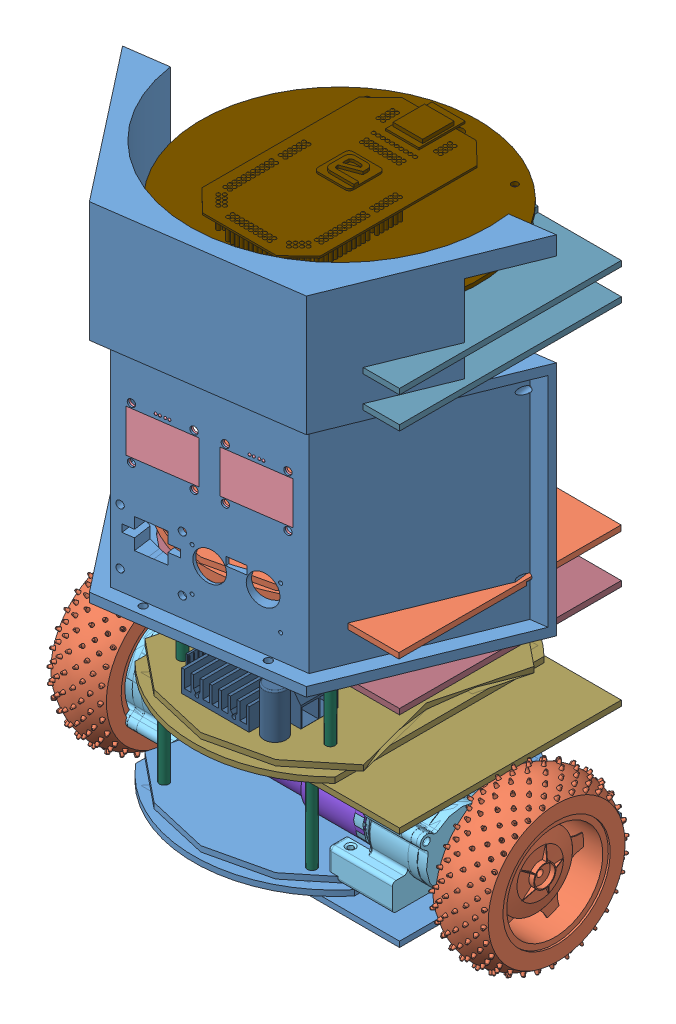
SolidWorks assembly Assembly_Final, configuration Default. Lengths in mm.
Overall size (236.68 351.62 182.38).
53 component instances, 26 part files, 124 mates.
Components (placement in the parent):
- BASE PLATE COMPACT-1: BASE PLATE COMPACT [Default] at (49.4415 46.8025 149.989) size (151.66 9 157.59)
- 85mm_Wheel-1: 85mm_Wheel [Default] at (-6.3675 60.3759 90.7884) x (0 -0.941771 -0.336255) z (0 0.336255 -0.941771) size (89.76 30.03 89.76)
- Bearing_large-1: Bearing_large [Default] at (14.6025 60.3759 90.7884) x (0 0 1) z (-1 0 0) size (34 34 10)
- Bearing_Modifiable-1: Bearing_Modifiable [Default] at (157.8505 60.3759 90.7897) x (0 0.995431 -0.095482) z (1 0 0) size (16 16 5)
- Gear Box Covering - Modifiable-1: Gear Box Covering - Modifiable [Default] at (31.0325 60.3759 90.7884) x (0 -0.541121 0.840945) z (-1 0 0) size (87.3 57.46 46.55)
- Gear_Driven - LARGE-1: Gear_Driven - LARGE [Default] at (169.8505 60.3759 90.7897) x (0 0.167526 -0.985868) z (1 0 0) size (41.92 41.92 47.93)
- Gear_Driver-1: Gear_Driver [Default] at (24.0325 76.7719 65.3077) x (0 0 1) z (-1 0 0) size (21.81 21.81 25.3)
- IG32 MOTORS-1: IG32 MOTORS [Default] at (41.0325 76.7719 65.3077) x (1 0 0) z (0 -1 0) size (92 51.5 40)
- LINE SENSOR-1: LINE SENSOR [Default] at (146.9415 49.8025 103.989) x (-1 0 0) z (0 0 1) size (100 13.5 28)
- Motor Driver-1: Motor Driver [Default] at (96.9415 105.8025 134.589) size (71 27 36.5)
- Motor_Main_Shaft-1: Motor_Main_Shaft [Default] at (41.0325 76.7719 65.3077) x (0 0 1) z (-1 0 0) size (6 6 15)
- Gear Box Covering - Modifiable-2: Gear Box Covering - Modifiable [Default] at (162.8505 60.3759 90.7897) x (0 -0.541121 -0.840945) z (1 0 0) size (87.3 57.46 46.55)
- Gear_Driver-2: Gear_Driver [Default] at (169.8505 76.7719 116.2703) x (0 -0.01238 -0.999923) z (1 0 0) size (21.81 21.81 25.3)
- Gear_Driven - LARGE-2: Gear_Driven - LARGE [Default] at (24.0325 60.3759 90.7884) x (0 0.762091 -0.64747) z (-1 0 0) size (41.92 41.92 47.93)
- IG32 MOTORS-2: IG32 MOTORS [Default] at (152.8505 76.7719 116.2703) x (-1 0 0) z (0 -1 0) size (92 51.5 40)
- Motor_Main_Shaft-2: Motor_Main_Shaft [Default] at (152.8505 76.7719 116.2703) x (0 -0.01238 -0.999923) z (1 0 0) size (6 6 15)
- Bearing_Modifiable-2: Bearing_Modifiable [Default] at (31.0325 60.3759 90.7884) x (0 0 -1) z (1 0 0) size (16 16 5)
- Bearing_Modifiable-3: Bearing_Modifiable [Default] at (14.6025 76.7719 65.3077) x (0 0 1) z (-1 0 0) size (16 16 5)
- Bearing_Modifiable-4: Bearing_Modifiable [Default] at (179.2805 76.7719 116.2703) x (0 0 -1) z (1 0 0) size (16 16 5)
- Bearing_large-2: Bearing_large [Default] at (179.2805 60.3759 90.7897) x (0 0 -1) z (1 0 0) size (34 34 10)
- 85mm_Wheel-2: 85mm_Wheel [Default] at (200.2505 60.3759 90.7897) x (0 0.770023 0.638016) z (0 0.638016 -0.770023) size (89.76 30.03 89.76)
- Floor_Plates1-1: Floor_Plates1 [Default] at (49.4415 99.8025 149.989) size (151.66 9 157.59)
- Floor_Plates2-1: Floor_Plates2 [Default] at (49.4415 155.8025 149.989) size (151.66 9 150)
- Floor_Plates4_2-1: Floor_Plates4_2 [Default] at (49.4415 288.8025 149.989) size (151.66 11 150)
- 3cm_spacers-1: 3cm_spacers [Default] at (56.9415 112.8025 144.839) x (0.995934 0 0.090084) z (0 -1 0) size (5 5 55)
- 3cm_spacers-2: 3cm_spacers [Default] at (56.9415 112.8025 35.139) x (0.477251 0 0.878767) z (0 -1 0) size (5 5 55)
- 3cm_spacers-3: 3cm_spacers [Default] at (136.9415 112.8025 144.839) x (0.906468 0 -0.422275) z (0 -1 0) size (5 5 55)
- 3cm_spacers-4: 3cm_spacers [Default] at (136.9415 112.8025 35.139) x (-0.928661 0 -0.370929) z (0 -1 0) size (5 5 55)
- 3cm_spacers-5: 3cm_spacers [Default] at (56.9415 165.8025 134.839) x (-0.9484 0 0.317076) z (0 -1 0) size (5 5 55)
- 3cm_spacers-6: 3cm_spacers [Default] at (136.9415 165.8025 45.139) x (0.243331 0 0.969943) z (0 -1 0) size (5 5 55)
- 3cm_spacers-7: 3cm_spacers [Default] at (56.9415 165.8025 45.139) x (0.021183 0 -0.999776) z (0 -1 0) size (5 5 55)
- 3cm_spacers-8: 3cm_spacers [Default] at (136.9007 165.8025 134.839) x (0.022963 0 -0.999736) z (0 -1 0) size (5 5 55)
- Motor Driver-2: Motor Driver [Default] at (96.9415 105.8025 45.389) size (71 27 36.5)
- 6cm_spacers-1: 6cm_spacers [Default] at (67.4804 303.8025 130.3876) x (-0.877081 0 0.480343) z (0 -1 0) size (5 5 150)
- 6cm_spacers-2: 6cm_spacers [Default] at (126.4026 303.8025 130.3876) x (-0.604095 0 0.796913) z (0 -1 0) size (5 5 150)
- 6cm_spacers-3: 6cm_spacers [Default] at (126.4026 303.8025 49.5905) x (0.449735 0 -0.893162) z (0 -1 0) size (5 5 150)
- 6cm_spacers-4: 6cm_spacers [Default] at (67.4804 303.8025 49.5905) x (-0.570107 0 0.82157) z (0 -1 0) size (5 5 150)
- Floor_Plates4_2-2: Floor_Plates4_2 [Default] at (49.4415 305.8025 149.989) size (151.66 11 150)
- spacer 2cm-2: spacer 2cm [Default] at (56.9415 318.8025 35.139) x (1 0 0) z (0 -1 0) size (5 5 15)
- spacer 2cm-3: spacer 2cm [Default] at (56.9415 318.8025 144.839) x (1 0 0) z (0 -1 0) size (5 5 15)
- spacer 2cm-4: spacer 2cm [Default] at (136.9415 318.8025 144.839) x (1 0 0) z (0 -1 0) size (5 5 15)
- spacer 2cm-5: spacer 2cm [Default] at (136.9415 318.8025 35.139) x (-0.160784 0 0.98699) z (0 -1 0) size (5 5 15)
- eYFi_Mega-2: eYFi_Mega [Default] at (76.9415 330.8025 143.989) size (150 18 150)
- Cover_mid-1: Cover_mid [Default] at (96.9415 158.8025 89.989) size (207.85 128 180) (hidden)
- Cover_Top-1: Cover_Top [Default] at (96.9415 336.8025 89.989) x (1 0 0) z (0 -1 0) size (207.85 180 50) (hidden)
- Cover_Bottom-1: Cover_Bottom [Default] at (96.9415 153.8025 89.989) size (205.85 109.54 180) (hidden)
- Cover_Bottom-2: Cover_Bottom [Default] at (96.9415 155.8025 89.989) x (0.990267 0 -0.139181) z (0.139181 0 0.990267) size (205.85 109.54 180) (hidden)
- Cover_Front-1: Cover_Front [Default] at (96.9415 160.8025 89.989) x (0.990267 0 -0.139181) z (0.139181 0 0.990267) size (207.85 188 90)
- Cover_Back-1: Cover_Back [Default] at (96.9415 160.8025 89.989) x (0.990267 0 -0.139181) z (0.139181 0 0.990267) size (207.85 188 90) (hidden)
- Dead_weight-1: Dead_weight [Default] at (49.303 182.022 149.8791) x (0.999997 0 0.002311) z (-0.002311 0 0.999997) size (151.66 12 150)
- Lead_Screw-1: Lead_Screw [Default] at (96.9415 158.8025 89.989) x (-0.659999 0 -0.751266) z (0.751266 0 -0.659999) size (7.8 150 7.8)
- OLED-2: OLED [Default] at (130.4266 242.3025 166.5739) x (0.990267 0 -0.139181) z (0.139181 0 0.990267) size (35 33 8.5)
- OLED-3: OLED [Default] at (85.8646 242.3025 172.8371) x (0.990267 0 -0.139181) z (0.139181 0 0.990267) size (35 33 8.5)
Mates (geometry in assembly coordinates):
- Coincident4: coincident anti-aligned: plane of BASE PLATE COMPACT-1 through (167.7549 49.8025 89.989) normal (0 -1 0); plane of LINE SENSOR-1 through (146.9415 49.8025 103.989) normal (0 1 0)
- Concentric1: concentric anti-aligned: cylinder of BASE PLATE COMPACT-1 through (49.4415 57.8025 101.489) axis (0 -1 0) radius 1.711; cylinder of LINE SENSOR-1 through (49.4415 47.8025 101.489) axis (0 1 0) radius 1.5
- Concentric2: concentric anti-aligned: cylinder of BASE PLATE COMPACT-1 through (144.4415 57.8025 101.489) axis (0 -1 0) radius 1.711; cylinder of LINE SENSOR-1 through (144.4415 47.8025 101.489) axis (0 1 0) radius 1.5
- Coincident9: coincident anti-aligned: plane of IG32 MOTORS-1 through (41.0325 76.7719 65.3077) normal (-1 0 0); plane of Motor_Main_Shaft-1 through (41.0325 76.7719 65.3077) normal (1 0 0)
- Concentric6: concentric aligned: cylinder of IG32 MOTORS-1 through (38.0325 76.7719 65.3077) axis (1 0 0) radius 10.5; cylinder of Motor_Main_Shaft-1 through (26.0325 76.7719 65.3077) axis (1 0 0) radius 3
- Coincident10: coincident anti-aligned: plane of IG32 MOTORS-2 through (152.8505 76.7719 116.2703) normal (1 0 0); plane of Motor_Main_Shaft-2 through (152.8505 76.7719 116.2703) normal (-1 0 0)
- Concentric7: concentric aligned: cylinder of IG32 MOTORS-2 through (155.8505 76.7719 116.2703) axis (-1 0 0) radius 10.5; cylinder of Motor_Main_Shaft-2 through (167.8505 76.7719 116.2703) axis (-1 0 0) radius 3
- Coincident11: coincident anti-aligned: plane of BASE PLATE COMPACT-1 through (167.7549 52.8025 89.989) normal (0 1 0); plane of Gear Box Covering - Modifiable-2 through (177.8505 52.8025 90.7897) normal (0 -1 0)
- Concentric8: concentric aligned: cylinder of BASE PLATE COMPACT-1 through (149.6005 41.8025 136.5916) axis (0 1 0) radius 1.75; cylinder of Gear Box Covering - Modifiable-2 through (149.6005 42.6025 136.5916) axis (0 1 0) radius 1.5
- Parallel5: parallel aligned: plane of BASE PLATE COMPACT-1 through (156.1015 49.8025 43.8903) normal (1 0 0); plane of Gear Box Covering - Modifiable-2 through (162.8505 76.7719 116.2703) normal (1 0 0)
- Coincident13: coincident anti-aligned: plane of BASE PLATE COMPACT-1 through (167.7549 52.8025 89.989) normal (0 1 0); plane of Gear Box Covering - Modifiable-1 through (16.0325 52.8025 90.7884) normal (0 -1 0)
- Concentric12: concentric aligned: cylinder of BASE PLATE COMPACT-1 through (44.2825 41.8025 44.9864) axis (0 1 0) radius 1.75; cylinder of Gear Box Covering - Modifiable-1 through (44.2825 42.6025 44.9864) axis (0 1 0) radius 1.5
- Parallel6: parallel aligned: plane of BASE PLATE COMPACT-1 through (37.7815 49.8025 43.8903) normal (-1 0 0); plane of Gear Box Covering - Modifiable-1 through (31.0325 76.7719 65.3077) normal (-1 0 0)
- Concentric13: concentric anti-aligned: cylinder of Gear Box Covering - Modifiable-2 through (167.8505 76.7719 116.2703) axis (-1 0 0) radius 10.75; cylinder of IG32 MOTORS-2 through (147.8505 76.7719 116.2703) axis (1 0 0) radius 16.5
- Concentric14: concentric aligned: cylinder of Gear Box Covering - Modifiable-2 through (157.8505 90.2719 116.2703) axis (1 0 0) radius 1.75; cylinder of IG32 MOTORS-2 through (149.8505 90.2719 116.2703) axis (1 0 0) radius 1.5
- Coincident16: coincident anti-aligned: plane of Gear Box Covering - Modifiable-2 through (152.8505 76.7719 116.2703) normal (-1 0 0); plane of IG32 MOTORS-2 through (152.8505 76.7719 116.2703) normal (1 0 0)
- Concentric15: concentric anti-aligned: cylinder of Gear Box Covering - Modifiable-1 through (26.0325 76.7719 65.3077) axis (1 0 0) radius 10.75; cylinder of IG32 MOTORS-1 through (46.0325 76.7719 65.3077) axis (-1 0 0) radius 16.5
- Concentric16: concentric aligned: cylinder of Gear Box Covering - Modifiable-1 through (36.0325 90.2719 65.3077) axis (-1 0 0) radius 1.75; cylinder of IG32 MOTORS-1 through (44.0325 90.2719 65.3077) axis (-1 0 0) radius 1.5
- Coincident17: coincident anti-aligned: plane of Gear Box Covering - Modifiable-1 through (41.0325 76.7719 65.3077) normal (1 0 0); plane of IG32 MOTORS-1 through (41.0325 76.7719 65.3077) normal (-1 0 0)
- Concentric17: concentric anti-aligned: cone of Gear_Driver-2 through (158.0485 76.7719 116.2703) axis (1 0 0); cylinder of Motor_Main_Shaft-2 through (167.8505 76.7719 116.2703) axis (-1 0 0) radius 3
- Concentric18: concentric anti-aligned: cylinder of Gear_Driver-2 through (161.8505 89.7709 116.1094) axis (0 -0.999923 0.01238) radius 2; cylinder of Motor_Main_Shaft-2 through (161.8505 73.2721 116.3136) axis (0 0.999923 -0.01238) radius 1.5
- Concentric19: concentric anti-aligned: cylinder of Gear_Driven - LARGE-1 through (154.9205 60.3759 90.7897) axis (1 0 0) radius 2.8; cylinder of Gear Box Covering - Modifiable-2 through (189.2805 60.3759 90.7897) axis (-1 0 0) radius 17.25
- Coincident18: coincident aligned: plane of Gear_Driven - LARGE-1 through (172.3505 60.3759 90.7897) normal (1 0 0); plane of Gear_Driver-2 through (172.3505 76.7719 116.2703) normal (1 0 0)
- Concentric20: concentric anti-aligned: cylinder of Gear_Driver-1 through (38.0325 76.7719 65.3077) axis (-1 0 0) radius 5.75; cylinder of Motor_Main_Shaft-1 through (26.0325 76.7719 65.3077) axis (1 0 0) radius 3
- Concentric21: concentric anti-aligned: cylinder of Gear_Driver-1 through (32.0325 89.7719 65.3077) axis (0 -1 0) radius 2; cylinder of Motor_Main_Shaft-1 through (32.0325 73.2719 65.3077) axis (0 1 0) radius 1.5
- Concentric24: concentric aligned: cylinder of Gear Box Covering - Modifiable-1 through (14.6025 60.3759 90.7884) axis (1 0 0) radius 22; cylinder of Gear_Driven - LARGE-2 through (-4.7675 60.3759 90.7884) axis (1 0 0) radius 7.5
- Coincident20: coincident aligned: plane of Gear_Driver-1 through (21.5325 76.7719 65.3077) normal (-1 0 0); plane of Gear_Driven - LARGE-2 through (21.5325 60.3759 90.7884) normal (-1 0 0)
- Concentric25: concentric anti-aligned: cylinder of Gear Box Covering - Modifiable-1 through (36.0325 60.3759 90.7884) axis (-1 0 0) radius 8.75; cylinder of Bearing_Modifiable-2 through (31.0325 60.3759 90.7884) axis (1 0 0) radius 8
- Coincident21: coincident aligned: plane of Gear Box Covering - Modifiable-1 through (31.0325 76.7719 65.3077) normal (-1 0 0); circle of Bearing_Modifiable-2
- Concentric27: concentric anti-aligned: cylinder of Gear Box Covering - Modifiable-1 through (9.6025 76.7719 65.3077) axis (1 0 0) radius 8.25; cylinder of Bearing_Modifiable-3 through (14.6025 76.7719 65.3077) axis (-1 0 0) radius 8
- Coincident22: coincident: line of Gear Box Covering - Modifiable-1 through (9.6025 62.7096 52.5308) axis (0 -0.672473 0.740122); plane of Bearing_Modifiable-3 through (9.6025 76.7719 65.3077) normal (-1 0 0)
- Concentric28: concentric anti-aligned: cylinder of Bearing_Modifiable-1 through (157.8505 60.3759 90.7897) axis (1 0 0) radius 8; cylinder of Gear Box Covering - Modifiable-2 through (189.2805 60.3759 90.7897) axis (-1 0 0) radius 17.25
- Coincident23: coincident aligned: plane of Bearing_Modifiable-1 through (162.8505 60.3759 90.7897) normal (1 0 0); plane of Gear Box Covering - Modifiable-2 through (162.8505 76.7719 116.2703) normal (1 0 0)
- Concentric30: concentric anti-aligned: cylinder of Gear Box Covering - Modifiable-2 through (184.2805 76.7719 116.2703) axis (-1 0 0) radius 8.25; cylinder of Bearing_Modifiable-4 through (179.2805 76.7719 116.2703) axis (1 0 0) radius 8
- Coincident25: coincident aligned: plane of Gear Box Covering - Modifiable-2 through (184.2805 83.1136 136.2899) normal (1 0 0); plane of Bearing_Modifiable-4 through (184.2805 76.7719 116.2703) normal (1 0 0)
- Concentric31: concentric anti-aligned: cylinder of Gear_Driven - LARGE-1 through (198.6505 60.3759 90.7897) axis (-1 0 0) radius 7.5; cylinder of Bearing_large-2 through (179.2805 60.3759 90.7897) axis (1 0 0) radius 17
- Coincident26: coincident aligned: plane of Gear Box Covering - Modifiable-2 through (189.2805 60.3759 90.7897) normal (1 0 0); plane of Bearing_large-2 through (189.2805 60.3759 90.7897) normal (1 0 0)
- Concentric32: concentric anti-aligned: cylinder of Bearing_large-1 through (14.6025 60.3759 90.7884) axis (-1 0 0) radius 17; cylinder of Gear_Driven - LARGE-2 through (-4.7675 60.3759 90.7884) axis (1 0 0) radius 7.5
- Coincident27: coincident aligned: plane of Bearing_large-1 through (4.6025 60.3759 90.7884) normal (-1 0 0); plane of Gear Box Covering - Modifiable-1 through (4.6025 60.3759 90.7884) normal (-1 0 0)
- Concentric33: concentric aligned: cylinder of Gear_Driven - LARGE-1 through (198.6505 60.3759 90.7897) axis (-1 0 0) radius 7.5; cylinder of 85mm_Wheel-2 through (208.8505 60.3759 90.7897) axis (-1 0 0) radius 5.5
- Coincident28: coincident anti-aligned: plane of Gear_Driven - LARGE-1 through (202.8505 64.8101 85.438) normal (0 0.937549 -0.347852); plane of 85mm_Wheel-2 through (198.6505 67.2277 91.954) normal (0 -0.937549 0.347852)
- Coincident29: coincident anti-aligned: plane of Gear_Driven - LARGE-1 through (202.8505 60.3759 90.7897) normal (1 0 0); plane of 85mm_Wheel-2 through (202.8505 60.3759 90.7897) normal (-1 0 0)
- Concentric34: concentric aligned: cylinder of 85mm_Wheel-1 through (-14.9675 60.3759 90.7884) axis (1 0 0) radius 5.5; cylinder of Gear_Driven - LARGE-2 through (-4.7675 60.3759 90.7884) axis (1 0 0) radius 7.5
- Coincident30: coincident anti-aligned: plane of 85mm_Wheel-1 through (-4.7675 55.876 85.4918) normal (0 0.17968 0.983725); plane of Gear_Driven - LARGE-2 through (-8.9675 62.7129 84.2431) normal (0 -0.17968 -0.983725)
- Coincident31: coincident anti-aligned: plane of 85mm_Wheel-1 through (-8.9675 60.3759 90.7884) normal (1 0 0); plane of Gear_Driven - LARGE-2 through (-8.9675 60.3759 90.7884) normal (-1 0 0)
- Concentric36: concentric anti-aligned: cylinder of BASE PLATE COMPACT-1 through (56.9415 59.8025 144.839) axis (0 -1 0) radius 1.25; cylinder of 3cm_spacers-1 through (56.9415 52.8025 144.839) axis (0 1 0) radius 2.5
- Coincident34: coincident anti-aligned: plane of BASE PLATE COMPACT-1 through (167.7549 52.8025 89.989) normal (0 1 0); circle of 3cm_spacers-1
- Concentric37: concentric anti-aligned: cylinder of BASE PLATE COMPACT-1 through (136.9415 59.8025 144.839) axis (0 -1 0) radius 1.25; cylinder of 3cm_spacers-3 through (136.9415 52.8025 144.839) axis (0 1 0) radius 2.5
- Coincident35: coincident anti-aligned: plane of BASE PLATE COMPACT-1 through (167.7549 52.8025 89.989) normal (0 1 0); plane of 3cm_spacers-3 through (136.9415 52.8025 144.839) normal (0 -1 0)
- Concentric38: concentric anti-aligned: cylinder of BASE PLATE COMPACT-1 through (136.9415 59.8025 35.139) axis (0 -1 0) radius 1.25; cylinder of 3cm_spacers-4 through (136.9415 52.8025 35.139) axis (0 1 0) radius 2.5
- Coincident36: coincident anti-aligned: plane of BASE PLATE COMPACT-1 through (167.7549 52.8025 89.989) normal (0 1 0); plane of 3cm_spacers-4 through (136.9415 52.8025 35.139) normal (0 -1 0)
- Concentric39: concentric anti-aligned: cylinder of BASE PLATE COMPACT-1 through (56.9415 59.8025 35.139) axis (0 -1 0) radius 1.25; cylinder of 3cm_spacers-2 through (56.9415 52.8025 35.139) axis (0 1 0) radius 2.5
- Coincident38: coincident anti-aligned: plane of BASE PLATE COMPACT-1 through (167.7549 52.8025 89.989) normal (0 1 0); plane of 3cm_spacers-2 through (56.9415 52.8025 35.139) normal (0 -1 0)
- Concentric40: concentric anti-aligned: cylinder of Floor_Plates1-1 through (136.9415 112.8025 144.839) axis (0 -1 0) radius 1.25; cylinder of 3cm_spacers-3 through (136.9415 52.8025 144.839) axis (0 1 0) radius 2.5
- Concentric41: concentric anti-aligned: cylinder of Floor_Plates1-1 through (56.9415 112.8025 35.139) axis (0 -1 0) radius 1.25; cylinder of 3cm_spacers-2 through (56.9415 52.8025 35.139) axis (0 1 0) radius 2.5
- Coincident39: coincident anti-aligned: plane of Floor_Plates1-1 through (167.7549 102.8025 89.989) normal (0 -1 0); plane of 3cm_spacers-2 through (56.9415 102.8025 35.139) normal (0 1 0)
- Concentric42: concentric anti-aligned: cylinder of Floor_Plates1-1 through (136.9007 112.8025 134.839) axis (0 -1 0) radius 1.5; cylinder of 3cm_spacers-8 through (136.9007 105.8025 134.839) axis (0 1 0) radius 2.5
- Concentric43: concentric anti-aligned: cylinder of Floor_Plates1-1 through (56.9415 112.8025 134.839) axis (0 -1 0) radius 1.5; cylinder of 3cm_spacers-5 through (56.9415 105.8025 134.839) axis (0 1 0) radius 2.5
- Concentric44: concentric anti-aligned: cylinder of Floor_Plates1-1 through (136.9415 112.8025 45.139) axis (0 -1 0) radius 1.5; axis of 3cm_spacers-6 through (136.9415 105.8025 45.139) axis (0 1 0)
- Concentric45: concentric anti-aligned: cylinder of Floor_Plates1-1 through (56.9415 112.8025 45.139) axis (0 -1 0) radius 1.5; cylinder of 3cm_spacers-7 through (56.9415 105.8025 45.139) axis (0 1 0) radius 2.5
- Coincident40: coincident anti-aligned: plane of Floor_Plates1-1 through (167.7549 105.8025 89.989) normal (0 1 0); plane of 3cm_spacers-5 through (56.9415 105.8025 134.839) normal (0 -1 0)
- Coincident41: coincident anti-aligned: plane of Floor_Plates1-1 through (167.7549 105.8025 89.989) normal (0 1 0); plane of 3cm_spacers-8 through (136.9007 105.8025 134.839) normal (0 -1 0)
- Coincident42: coincident anti-aligned: plane of Floor_Plates1-1 through (167.7549 105.8025 89.989) normal (0 1 0); plane of 3cm_spacers-7 through (56.9415 105.8025 45.139) normal (0 -1 0)
- Coincident43: coincident anti-aligned: plane of Floor_Plates1-1 through (167.7549 105.8025 89.989) normal (0 1 0); circle of 3cm_spacers-6
- Coincident44: coincident anti-aligned: plane of Floor_Plates2-1 through (96.9415 155.8025 89.989) normal (0 -1 0); plane of 3cm_spacers-7 through (56.9415 155.8025 45.139) normal (0 1 0)
- Concentric48: concentric aligned: cylinder of Floor_Plates2-1 through (56.9415 148.8025 45.139) axis (0 1 0) radius 1.5; cylinder of 3cm_spacers-7 through (56.9415 105.8025 45.139) axis (0 1 0) radius 2.5
- Concentric49: concentric aligned: cylinder of Floor_Plates2-1 through (56.9415 148.8025 134.839) axis (0 1 0) radius 1.5; cylinder of 3cm_spacers-5 through (56.9415 150.8025 134.839) axis (0 1 0) radius 1.25
- Concentric50: concentric aligned: cylinder of Floor_Plates2-1 through (67.4804 148.8025 130.3876) axis (0 1 0) radius 1.5; cylinder of 6cm_spacers-1 through (67.4804 158.8025 130.3876) axis (0 1 0) radius 2.5
- Concentric51: concentric aligned: cylinder of Floor_Plates2-1 through (126.4026 148.8025 130.3876) axis (0 1 0) radius 1.5; cylinder of 6cm_spacers-2 through (126.4026 158.8025 130.3876) axis (0 1 0) radius 2.5
- Concentric52: concentric aligned: cylinder of Floor_Plates2-1 through (126.4026 148.8025 49.5905) axis (0 1 0) radius 1.5; cylinder of 6cm_spacers-3 through (126.4026 158.8025 49.5905) axis (0 1 0) radius 2.5
- Concentric53: concentric aligned: cylinder of Floor_Plates2-1 through (67.4804 148.8025 49.5905) axis (0 1 0) radius 1.5; cylinder of 6cm_spacers-4 through (67.4804 158.8025 49.5905) axis (0 1 0) radius 2.5
- Coincident45: coincident anti-aligned: plane of Floor_Plates2-1 through (96.9415 158.8025 89.989) normal (0 1 0); plane of 6cm_spacers-4 through (67.4804 158.8025 49.5905) normal (0 -1 0)
- Coincident46: coincident anti-aligned: plane of Floor_Plates2-1 through (96.9415 158.8025 89.989) normal (0 1 0); circle of 6cm_spacers-3
- Coincident47: coincident anti-aligned: plane of Floor_Plates2-1 through (96.9415 158.8025 89.989) normal (0 1 0); plane of 6cm_spacers-2 through (126.4026 158.8025 130.3876) normal (0 -1 0)
- Coincident48: coincident anti-aligned: plane of Floor_Plates2-1 through (96.9415 158.8025 89.989) normal (0 1 0); plane of 6cm_spacers-1 through (67.4804 158.8025 130.3876) normal (0 -1 0)
- Concentric54: concentric aligned: cylinder of Floor_Plates2-1 through (96.9415 155.8025 89.989) axis (0 1 0) radius 75; cylinder of Floor_Plates4_2-1 through (96.9415 286.8025 89.989) axis (0 1 0) radius 75
- Concentric55: concentric anti-aligned: cylinder of Floor_Plates4_2-1 through (126.4026 296.8025 130.3876) axis (0 -1 0) radius 1.5; cylinder of 6cm_spacers-2 through (126.4026 158.8025 130.3876) axis (0 1 0) radius 2.5
- Concentric57: concentric aligned: cylinder of Floor_Plates4_2-1 through (96.9415 281.8025 89.989) axis (0 1 0) radius 8.4; cylinder of Floor_Plates4_2-2 through (96.9415 298.8025 89.989) axis (0 1 0) radius 8.4
- Concentric58: concentric aligned: cylinder of Floor_Plates4_2-1 through (156.9415 281.8025 89.989) axis (0 1 0) radius 8.4; cylinder of Floor_Plates4_2-2 through (156.9415 298.8025 89.989) axis (0 1 0) radius 8.4
- Coincident51: coincident anti-aligned: plane of 6cm_spacers-2 through (126.4026 303.8025 130.3876) normal (0 1 0); plane of Floor_Plates4_2-2 through (96.9415 303.8025 89.989) normal (0 -1 0)
- Concentric59: concentric anti-aligned: cylinder of Floor_Plates4_2-2 through (56.9415 318.8025 35.139) axis (0 -1 0) radius 1.25; cylinder of spacer 2cm-2 through (56.9415 308.8025 35.139) axis (0 1 0) radius 2.5
- Concentric60: concentric anti-aligned: cylinder of Floor_Plates4_2-2 through (136.9415 318.8025 35.139) axis (0 -1 0) radius 1.25; cylinder of spacer 2cm-5 through (136.9415 308.8025 35.139) axis (0 1 0) radius 2.5
- Concentric61: concentric anti-aligned: cylinder of Floor_Plates4_2-2 through (136.9415 318.8025 144.839) axis (0 -1 0) radius 1.25; cylinder of spacer 2cm-4 through (136.9415 308.8025 144.839) axis (0 1 0) radius 2.5
- Concentric62: concentric anti-aligned: cylinder of Floor_Plates4_2-2 through (56.9415 318.8025 144.839) axis (0 -1 0) radius 1.25; cylinder of spacer 2cm-3 through (56.9415 308.8025 144.839) axis (0 1 0) radius 2.5
- Coincident52: coincident anti-aligned: plane of Floor_Plates4_2-2 through (96.9415 308.8025 89.989) normal (0 1 0); plane of spacer 2cm-3 through (56.9415 308.8025 144.839) normal (0 -1 0)
- Coincident53: coincident anti-aligned: plane of Floor_Plates4_2-2 through (96.9415 308.8025 89.989) normal (0 1 0); circle of spacer 2cm-4
- Coincident54: coincident anti-aligned: plane of Floor_Plates4_2-2 through (96.9415 308.8025 89.989) normal (0 1 0); plane of spacer 2cm-5 through (136.9415 308.8025 35.139) normal (0 -1 0)
- Coincident55: coincident anti-aligned: plane of Floor_Plates4_2-2 through (96.9415 308.8025 89.989) normal (0 1 0); plane of spacer 2cm-2 through (56.9415 308.8025 35.139) normal (0 -1 0)
- Coincident58: coincident anti-aligned: plane of spacer 2cm-2 through (56.9415 318.8025 35.139) normal (0 1 0); plane of eYFi_Mega-2 through (96.9415 318.8025 89.989) normal (0 -1 0)
- Concentric64: concentric aligned: cylinder of Floor_Plates4_2-2 through (96.9415 303.8025 89.989) axis (0 1 0) radius 75; cylinder of eYFi_Mega-2 through (96.9415 318.8025 89.989) axis (0 1 0) radius 75
- Parallel12: parallel aligned: cylinder of spacer 2cm-2 through (56.9415 308.8025 35.139) axis (0 1 0) radius 2.5; cylinder of eYFi_Mega-2 through (56.9415 310.8025 35.089) axis (0 1 0) radius 1.75
- Parallel15: parallel aligned: cylinder of spacer 2cm-4 through (136.9415 313.8025 144.839) axis (0 1 0) radius 1.5; cylinder of eYFi_Mega-2 through (136.9415 310.8025 144.889) axis (0 1 0) radius 1.75
- Coincident59: coincident anti-aligned: plane of Floor_Plates1-1 through (167.7549 105.8025 89.989) normal (0 1 0); plane of Motor Driver-2 through (96.9415 105.8025 45.389) normal (0 -1 0)
- Coincident60: coincident anti-aligned: plane of Motor Driver-1 through (96.9415 105.8025 134.589) normal (0 -1 0); plane of Floor_Plates1-1 through (167.7549 105.8025 89.989) normal (0 1 0)
- Concentric71: concentric anti-aligned: cylinder of Motor Driver-1 through (64.4415 105.8025 149.839) axis (0 1 0) radius 1.5; cylinder of Floor_Plates1-1 through (64.4415 112.8025 149.839) axis (0 -1 0) radius 1.5
- Concentric72: concentric anti-aligned: cylinder of Floor_Plates1-1 through (64.4415 112.8025 30.139) axis (0 -1 0) radius 1.5; cylinder of Motor Driver-2 through (64.4415 105.8025 30.139) axis (0 1 0) radius 1.5
- Concentric73: concentric anti-aligned: cylinder of Floor_Plates4_2-1 through (96.9415 286.8025 89.989) axis (0 1 0) radius 75; cylinder of Cover_mid-1 through (96.9415 281.8025 89.989) axis (0 -1 0) radius 79
- Parallel16: parallel: line of eYFi_Mega-2 through (76.9415 331.8025 143.989) axis (1 0 0); plane of Cover_mid-1 through (44.98 286.8025 179.989) normal (0 0 1)
- Coincident62: coincident anti-aligned: plane of Floor_Plates2-1 through (96.9415 158.8025 89.989) normal (0 1 0); plane of Cover_mid-1 through (96.9415 158.8025 89.989) normal (0 -1 0)
- Coincident63: coincident anti-aligned: plane of Floor_Plates4_2-1 through (96.9415 286.8025 89.989) normal (0 -1 0); plane of Cover_mid-1 through (96.9415 286.8025 89.989) normal (0 1 0)
- Coincident64: coincident aligned: plane of Cover_mid-1 through (44.98 286.8025 179.989) normal (0 0 1); plane of Cover_Bottom-1 through (44.98 158.8025 179.989) normal (0 0 1)
- Concentric74: concentric aligned: cylinder of eYFi_Mega-2 through (96.9415 318.8025 89.989) axis (0 1 0) radius 75; cylinder of Cover_Bottom-1 through (96.9415 53.8025 89.989) axis (0 1 0) radius 79
- Coincident65: coincident anti-aligned: plane of Cover_mid-1 through (96.9415 158.8025 89.989) normal (0 -1 0); plane of Cover_Bottom-1 through (96.9415 158.8025 89.989) normal (0 1 0)
- Concentric77: concentric aligned: cylinder of Floor_Plates4_2-2 through (96.9415 303.8025 89.989) axis (0 1 0) radius 75; cylinder of Cover_Top-1 through (96.9415 286.8025 89.989) axis (0 1 0) radius 76
- Parallel19: parallel aligned: plane of Cover_mid-1 through (44.98 286.8025 179.989) normal (0 0 1); plane of Cover_Top-1 through (148.9031 286.8025 179.989) normal (0 0 1)
- Coincident70: coincident anti-aligned: plane of Cover_mid-1 through (96.9415 286.8025 89.989) normal (0 1 0); plane of Cover_Top-1 through (96.9415 286.8025 89.989) normal (0 -1 0)
- Parallel22: parallel aligned: plane of BASE PLATE COMPACT-1 through (156.1015 49.8025 43.8903) normal (1 0 0); plane of Cover_Bottom-1 through (199.8646 148.8025 89.989) normal (1 0 0)
- Concentric78: concentric aligned: cylinder of Floor_Plates2-1 through (96.9415 163.8025 89.989) axis (0 -1 0) radius 8.35; cylinder of Cover_Front-1 through (96.9415 283.8025 89.989) axis (0 -1 0) radius 81
- Concentric79: concentric aligned: cylinder of Floor_Plates2-1 through (96.9415 163.8025 89.989) axis (0 -1 0) radius 8.35; cylinder of Cover_Back-1 through (96.9415 283.8025 89.989) axis (0 -1 0) radius 81
- Coincident72: coincident anti-aligned: plane of Floor_Plates2-1 through (96.9415 155.8025 89.989) normal (0 -1 0); plane of Cover_Bottom-2 through (96.9415 155.8025 89.989) normal (0 1 0)
- Concentric80: concentric anti-aligned: cylinder of Floor_Plates2-1 through (96.9415 163.8025 89.989) axis (0 -1 0) radius 25; cylinder of Cover_Bottom-2 through (96.9415 55.8025 89.989) axis (0 1 0) radius 79
- Coincident73: coincident anti-aligned: plane of Cover_Bottom-2 through (96.9415 160.8025 89.989) normal (0 1 0); plane of Cover_Front-1 through (96.9415 160.8025 89.989) normal (0 -1 0)
- Coincident74: coincident aligned: plane of Cover_Bottom-2 through (160.9236 160.8025 171.881) normal (0.927187 0 0.374599); plane of Cover_Front-1 through (180.3884 165.8025 123.7029) normal (0.927187 0 0.374599)
- Coincident75: coincident anti-aligned: plane of Cover_Bottom-2 through (96.9415 160.8025 89.989) normal (0 1 0); plane of Cover_Back-1 through (96.9415 160.8025 89.989) normal (0 -1 0)
- Coincident76: coincident aligned: plane of Cover_Bottom-2 through (199.8531 160.8025 75.5249) normal (0.788006 0 -0.615668); plane of Cover_Back-1 through (199.8531 165.8025 75.5249) normal (0.788006 0 -0.615668)
- Concentric81: concentric anti-aligned: cylinder of Floor_Plates2-1 through (96.9415 163.8025 89.989) axis (0 -1 0) radius 8.35; cylinder of Dead_weight-1 through (96.9415 180.022 89.989) axis (0 1 0) radius 72.5
- Concentric82: concentric aligned: cylinder of Floor_Plates2-1 through (96.9415 163.8025 89.989) axis (0 -1 0) radius 25; cylinder of Lead_Screw-1 through (96.9415 308.8025 89.989) axis (0 -1 0) radius 3.9
- Coincident77: coincident anti-aligned: plane of Floor_Plates2-1 through (96.9415 158.8025 89.989) normal (0 1 0); plane of Lead_Screw-1 through (96.9415 158.8025 89.989) normal (0 -1 0)
- Concentric83: concentric anti-aligned: cylinder of Cover_Front-1 through (144.1672 256.3025 156.5641) axis (0.139181 0 0.990267) radius 2; cylinder of OLED-2 through (145.4198 256.3025 165.4765) axis (-0.139181 0 -0.990267) radius 2
- Concentric84: concentric anti-aligned: cylinder of Cover_Front-1 through (114.4592 228.3025 160.7395) axis (0.139181 0 0.990267) radius 2; cylinder of OLED-2 through (115.7118 228.3025 169.6519) axis (-0.139181 0 -0.990267) radius 2
- Coincident83: coincident anti-aligned: plane of Cover_Front-1 through (108.2848 160.8025 170.6958) normal (-0.139181 0 -0.990267); plane of OLED-2 through (130.5658 242.3025 167.5642) normal (0.139181 0 0.990267)
- Concentric85: concentric anti-aligned: cylinder of Cover_Front-1 through (99.6052 256.3025 162.8272) axis (0.139181 0 0.990267) radius 2; cylinder of OLED-3 through (100.8578 256.3025 171.7396) axis (-0.139181 0 -0.990267) radius 2
- Concentric86: concentric anti-aligned: cylinder of Cover_Front-1 through (69.8972 228.3025 167.0027) axis (0.139181 0 0.990267) radius 2; cylinder of OLED-3 through (71.1498 228.3025 175.9151) axis (-0.139181 0 -0.990267) radius 2
- Coincident84: coincident anti-aligned: plane of Cover_Front-1 through (108.2848 160.8025 170.6958) normal (-0.139181 0 -0.990267); plane of OLED-3 through (86.0038 242.3025 173.8273) normal (0.139181 0 0.990267)
